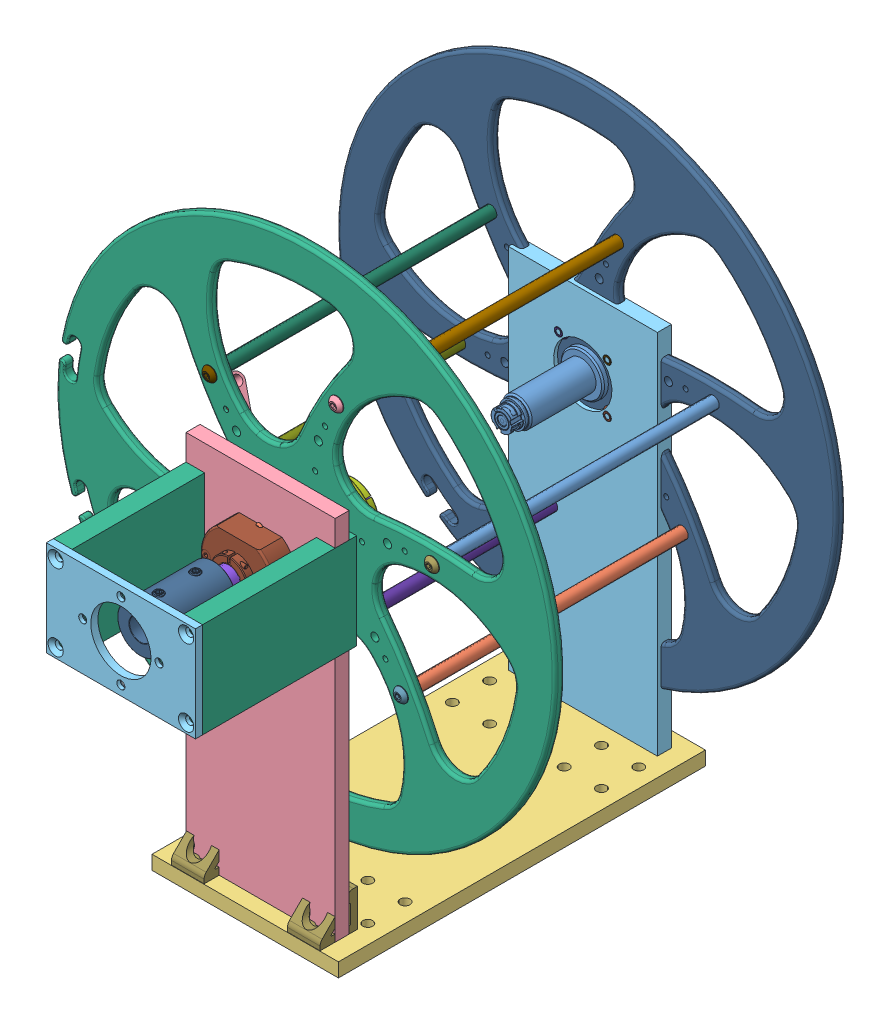
SolidWorks assembly Winch V2, configuration Default. Lengths in mm.
Overall size (340 379.53 358.94).
54 component instances, 48 part files, 0 mates.
Components (placement in the parent):
- Spool Support.step-1: Spool Support.step [Default] at (-13.1975 -9.525 242.4976) x (0 0 -1) z (1 0 0) size (250 259.52 127)
  - 5448T18.step-1: 5448T18.step [Default] at (-67.0274 209.525 13.1975) x (0 -1 0) z (0 0 1) size (23 16 23)
  - 92095A113.step-1: 92095A113.step [Default] at (-66.9844 229.525 13.1975) x (0 0 -1) z (-1 0 0) size (4.5 4.5 4.5)
  - 92095A113.step-2: 92095A113.step [Default] at (-66.9844 189.525 13.1975) x (0 0 -1) z (-1 0 0) size (4.5 4.5 4.5)
  - Spool Support-0.step-1: Spool Support-0.step [Default] at origin size (250 9.53 127)
  - Spool Support-1.step-1: Spool Support-1.step [Default] at origin size (9.53 250 101.6)
  - Spool Support-2.step-1: Spool Support-2.step [Default] at origin size (9.53 250 101.6)
- Spool Core.step-1: Spool Core.step [Default] at (13.4446 195.1511 -61.4824) x (0 1 0) z (0 0 1) size (340 340 240.83)
  - Component12.step-1: Component12.step [Default] at (-7.5076 6.2623 2.175) x (0.766044 -0.642788 0) z (0 0 1) size (9.5 9.5 14.75)
  - Component13.step-1: Component13.step [Default] at (-7.5076 6.2623 2.175) x (0.766044 -0.642788 0) z (0 0 1) size (9.5 9.5 14.75)
  - Component14.step-1: Component14.step [Default] at (-10.8225 46.1728 670.1648) x (1 0 0) z (0 0 -1) size (9.5 9.5 14.75)
  - Component15.step-1: Component15.step [Default] at (-7.5076 6.2623 2.175) x (0.766044 -0.642788 0) z (0 0 1) size (9.5 9.5 14.75)
  - Spool Core-3.step-1: Spool Core-3.step [Default] at origin size (340 340 6.35)
  - Spool Core-4.step-1: Spool Core-4.step [Default] at origin size (9.5 9.5 14.75)
  - Spool Core-5.step-1: Spool Core-5.step [Default] at origin size (8.18 8.18 9.12)
  - Spool Core-6.step-1: Spool Core-6.step [Default] at origin size (9.5 9.5 14.75)
  - Spool Core-7.step-1: Spool Core-7.step [Default] at origin size (9.5 9.5 14.75)
  - Spool Core-8.step-1: Spool Core-8.step [Default] at origin size (8 8 185)
  - Spool Core-9.step-1: Spool Core-9.step [Default] at origin size (8 8 185)
  - Spool Core-10.step-1: Spool Core-10.step [Default] at origin size (8 8 185)
  - Spool Core-11.step-1: Spool Core-11.step [Default] at origin size (9.5 9.5 14.75)
  - Spool Core-12.step-1: Spool Core-12.step [Default] at origin size (8 8 185)
  - Spool Core-13.step-1: Spool Core-13.step [Default] at origin size (8 8 185)
  - Spool Core-14.step-1: Spool Core-14.step [Default] at origin size (9.5 9.5 14.75)
  - Spool Core-15.step-1: Spool Core-15.step [Default] at origin size (9.5 9.5 14.75)
  - Spool Core-16.step-1: Spool Core-16.step [Default] at origin size (9.5 9.5 14.75)
  - Spool Core-17.step-1: Spool Core-17.step [Default] at origin size (340 340 6.35)
  - Spool Core-18.step-1: Spool Core-18.step [Default] at origin size (17.75 23.28 7.94)
  - Spool Core-19.step-1: Spool Core-19.step [Default] at origin size (9.5 9.5 14.75)
  - Spool Core-20.step-1: Spool Core-20.step [Default] at origin size (8 8 185)
  - Spool Core-21.step-1: Spool Core-21.step [Default] at origin size (23.39 18.02 7.94)
  - Spool Core-22.step-1: Spool Core-22.step [Default] at origin size (9.5 9.5 14.75)
  - Spool Core-23.step-1: Spool Core-23.step [Default] at origin size (9.5 9.5 14.75)
  - Spool Core-24.step-1: Spool Core-24.step [Default] at origin size (9.5 9.5 14.75)
  - Spool Core-25.step-1: Spool Core-25.step [Default] at origin size (9.5 9.5 14.75)
  - Spool Core-26.step-1: Spool Core-26.step [Default] at origin size (8.18 8.18 9.12)
  - Spool Core-27.step-1: Spool Core-27.step [Default] at origin size (9.5 9.5 14.75)
  - Spool Core-28.step-1: Spool Core-28.step [Default] at origin size (9.5 9.5 14.75)
  - Spool Core-29.step-1: Spool Core-29.step [Default] at origin size (9.5 9.5 14.75)
  - Spool Core-30.step-1: Spool Core-30.step [Default] at origin size (56 56 99.65)
  - Spool Core-31.step-1: Spool Core-31.step [Default] at origin size (8.18 8.18 9.12)
  - Spool Core-32.step-1: Spool Core-32.step [Default] at origin size (9.5 9.5 14.75)
  - Spool Core-33.step-1: Spool Core-33.step [Default] at origin size (23.71 23.42 7.94)
- Motor Support.step-1: Motor Support.step [Default] at (-17.8977 208.142 442.889) x (0 0 1) z (-1 0 0) size (109.83 65 101.6)
  - Component1.step-1: Component1.step [Default] at (-45 0 0) size (4.83 65 101.6)
  - Component2.step-1: Component2.step [Default] at (-7.2906 1.3024 20.2023) size (105 65 12.7)
  - Component2.step-2: Component2.step [Default] at (-7.2906 1.3024 -68.6977) size (105 65 12.7)
- Shaft Clamp.step-1: Shaft Clamp.step [Default] at (0 200 264.925) x (0.707107 0.707107 0) z (0 0 1) size (63 63 21)
- Shaft.step-1: Shaft.step [Default] at (0 200 257.525) size (16 16 118.4)
- Shaft Clamp Adapter.step-1: Shaft Clamp Adapter.step [Default] at (0 200 270.425) x (0 0 -1) z (0.707107 0.707107 0) size (6.35 68 68)
- Shaft Coupler.step-1: Shaft Coupler.step [Default] at (0 200 364.525) size (31 31.76 50.01)
- Encoder.step-1: Encoder.step [Default] at (0 200 304.36) x (1 0 0) z (0 0 -1) size (50.8 52.34 36.53)
- 47065T663.step-1: 47065T663.step [Default] at (39.6392 0 292.3608) x (0 0 1) z (-1 0 0) size (25.4 25.4 22.23)
- 47065T663.step-2: 47065T663.step [Default] at (-39.3608 0 292.3608) x (0 0 1) z (-1 0 0) size (25.4 25.4 22.23)
